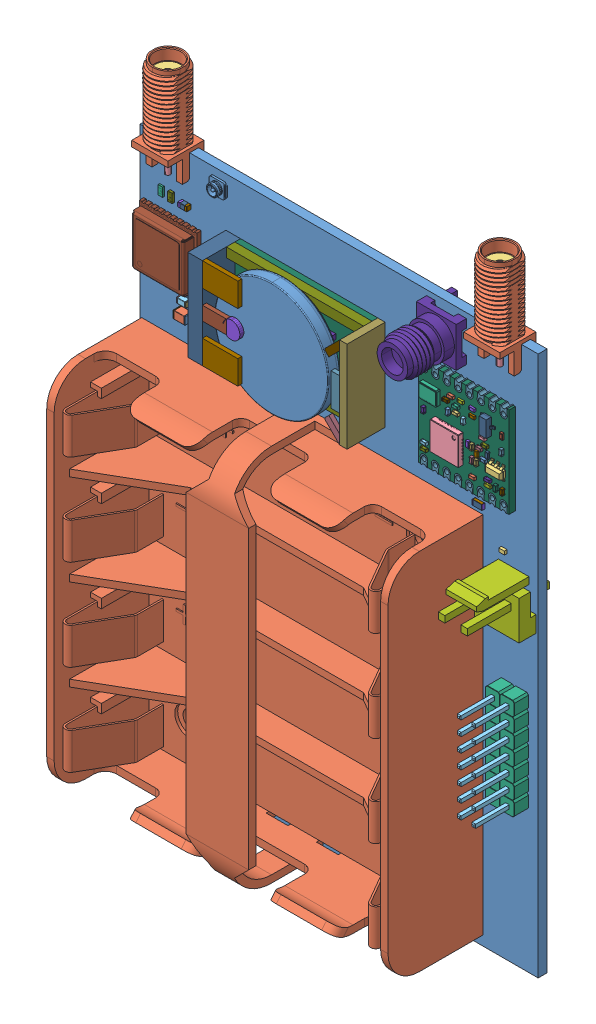
SolidWorks assembly Печатная плата Peggy Tracker, configuration Default. Lengths in mm. (continued)
Components (placement in the parent): (continued)
- Печатная плата Peggy Tracker(2)^Печатная плата Peggy Tracker-1: Печатная плата Peggy Tracker(2)^Печатная плата Peggy Tracker [Default] at origin size (70 108.1 20.64) (virtual) (continued)
  - MPU1^Печатная плата Peggy Tracker(2)_Печатная плата Peggy Tracker-1: MPU1^Печатная плата Peggy Tracker(2)_Печатная плата Peggy Tracker [Default] at origin size (12 12 1.2) (virtual) (continued)
    - 5945464032^MPU1_Печатная плата Peggy Tracker(2)_Печатная плата Peggy Tracker-1: 5945464032^MPU1_Печатная плата Peggy Tracker(2)_Печатная плата Peggy Tracker [Default] at (31.9001 39.0001 -1.5596) x (0 1 0) z (0 0 -1) size (12 12 1.2) (virtual) (continued)
      - Leader^5945464032_MPU1_Печатная плата Peggy Tracker(2)_Печатная плата Peggy Tracker-3: Leader^5945464032_MPU1_Печатная плата Peggy Tracker(2)_Печатная плата Peggy Tracker [По умолчанию] at (-5 -2.4 0) x (-1 0 0) z (0 0 1) size (1 0.38 0.68) (virtual)
      - Leader^5945464032_MPU1_Печатная плата Peggy Tracker(2)_Печатная плата Peggy Tracker-4: Leader^5945464032_MPU1_Печатная плата Peggy Tracker(2)_Печатная плата Peggy Tracker [По умолчанию] at (-5 -1.6 0) x (-1 0 0) z (0 0 1) size (1 0.38 0.68) (virtual)
      - Leader^5945464032_MPU1_Печатная плата Peggy Tracker(2)_Печатная плата Peggy Tracker-5: Leader^5945464032_MPU1_Печатная плата Peggy Tracker(2)_Печатная плата Peggy Tracker [По умолчанию] at (-5 -0.8 0) x (-1 0 0) z (0 0 1) size (1 0.38 0.68) (virtual)
      - Leader^5945464032_MPU1_Печатная плата Peggy Tracker(2)_Печатная плата Peggy Tracker-6: Leader^5945464032_MPU1_Печатная плата Peggy Tracker(2)_Печатная плата Peggy Tracker [По умолчанию] at (-5 0 0) x (-1 0 0) z (0 0 1) size (1 0.38 0.68) (virtual)
      - Leader^5945464032_MPU1_Печатная плата Peggy Tracker(2)_Печатная плата Peggy Tracker-7: Leader^5945464032_MPU1_Печатная плата Peggy Tracker(2)_Печатная плата Peggy Tracker [По умолчанию] at (-5 0.8 0) x (-1 0 0) z (0 0 1) size (1 0.38 0.68) (virtual)
      - Leader^5945464032_MPU1_Печатная плата Peggy Tracker(2)_Печатная плата Peggy Tracker-8: Leader^5945464032_MPU1_Печатная плата Peggy Tracker(2)_Печатная плата Peggy Tracker [По умолчанию] at (-5 1.6 0) x (-1 0 0) z (0 0 1) size (1 0.38 0.68) (virtual)
      - Leader^5945464032_MPU1_Печатная плата Peggy Tracker(2)_Печатная плата Peggy Tracker-9: Leader^5945464032_MPU1_Печатная плата Peggy Tracker(2)_Печатная плата Peggy Tracker [По умолчанию] at (-5 2.4 0) x (-1 0 0) z (0 0 1) size (1 0.38 0.68) (virtual)
      - Leader^5945464032_MPU1_Печатная плата Peggy Tracker(2)_Печатная плата Peggy Tracker-10: Leader^5945464032_MPU1_Печатная плата Peggy Tracker(2)_Печатная плата Peggy Tracker [По умолчанию] at (-5 3.2 0) x (-1 0 0) z (0 0 1) size (1 0.38 0.68) (virtual)
      - Leader^5945464032_MPU1_Печатная плата Peggy Tracker(2)_Печатная плата Peggy Tracker-11: Leader^5945464032_MPU1_Печатная плата Peggy Tracker(2)_Печатная плата Peggy Tracker [По умолчанию] at (-5 4 0) x (-1 0 0) z (0 0 1) size (1 0.38 0.68) (virtual)
      - Leader^5945464032_MPU1_Печатная плата Peggy Tracker(2)_Печатная плата Peggy Tracker-12: Leader^5945464032_MPU1_Печатная плата Peggy Tracker(2)_Печатная плата Peggy Tracker [По умолчанию] at (5 -4 0) size (1 0.38 0.68) (virtual)
      - Leader^5945464032_MPU1_Печатная плата Peggy Tracker(2)_Печатная плата Peggy Tracker-13: Leader^5945464032_MPU1_Печатная плата Peggy Tracker(2)_Печатная плата Peggy Tracker [По умолчанию] at (5 -3.2 0) size (1 0.38 0.68) (virtual)
      - Leader^5945464032_MPU1_Печатная плата Peggy Tracker(2)_Печатная плата Peggy Tracker-14: Leader^5945464032_MPU1_Печатная плата Peggy Tracker(2)_Печатная плата Peggy Tracker [По умолчанию] at (5 -2.4 0) size (1 0.38 0.68) (virtual)
      - Leader^5945464032_MPU1_Печатная плата Peggy Tracker(2)_Печатная плата Peggy Tracker-15: Leader^5945464032_MPU1_Печатная плата Peggy Tracker(2)_Печатная плата Peggy Tracker [По умолчанию] at (5 -1.6 0) size (1 0.38 0.68) (virtual)
      - Leader^5945464032_MPU1_Печатная плата Peggy Tracker(2)_Печатная плата Peggy Tracker-16: Leader^5945464032_MPU1_Печатная плата Peggy Tracker(2)_Печатная плата Peggy Tracker [По умолчанию] at (5 -0.8 0) size (1 0.38 0.68) (virtual)
      - Leader^5945464032_MPU1_Печатная плата Peggy Tracker(2)_Печатная плата Peggy Tracker-17: Leader^5945464032_MPU1_Печатная плата Peggy Tracker(2)_Печатная плата Peggy Tracker [По умолчанию] at (5 0 0) size (1 0.38 0.68) (virtual)
      - Leader^5945464032_MPU1_Печатная плата Peggy Tracker(2)_Печатная плата Peggy Tracker-18: Leader^5945464032_MPU1_Печатная плата Peggy Tracker(2)_Печатная плата Peggy Tracker [По умолчанию] at (5 0.8 0) size (1 0.38 0.68) (virtual)
      - Leader^5945464032_MPU1_Печатная плата Peggy Tracker(2)_Печатная плата Peggy Tracker-19: Leader^5945464032_MPU1_Печатная плата Peggy Tracker(2)_Печатная плата Peggy Tracker [По умолчанию] at (5 1.6 0) size (1 0.38 0.68) (virtual)
      - Leader^5945464032_MPU1_Печатная плата Peggy Tracker(2)_Печатная плата Peggy Tracker-20: Leader^5945464032_MPU1_Печатная плата Peggy Tracker(2)_Печатная плата Peggy Tracker [По умолчанию] at (5 2.4 0) size (1 0.38 0.68) (virtual)
      - Leader^5945464032_MPU1_Печатная плата Peggy Tracker(2)_Печатная плата Peggy Tracker-21: Leader^5945464032_MPU1_Печатная плата Peggy Tracker(2)_Печатная плата Peggy Tracker [По умолчанию] at (5 3.2 0) size (1 0.38 0.68) (virtual)
      - Leader^5945464032_MPU1_Печатная плата Peggy Tracker(2)_Печатная плата Peggy Tracker-22: Leader^5945464032_MPU1_Печатная плата Peggy Tracker(2)_Печатная плата Peggy Tracker [По умолчанию] at (5 4 0) size (1 0.38 0.68) (virtual)
      - Leader-13^5945464032_MPU1_Печатная плата Peggy Tracker(2)_Печатная плата Peggy Tracker-1: Leader-13^5945464032_MPU1_Печатная плата Peggy Tracker(2)_Печатная плата Peggy Tracker [По умолчанию] at (-4 -5 0) x (0 -1 0) z (0 0 1) size (1 0.38 0.68) (virtual)
      - Leader-13^5945464032_MPU1_Печатная плата Peggy Tracker(2)_Печатная плата Peggy Tracker-2: Leader-13^5945464032_MPU1_Печатная плата Peggy Tracker(2)_Печатная плата Peggy Tracker [По умолчанию] at (-3.2 -5 0) x (0 -1 0) z (0 0 1) size (1 0.38 0.68) (virtual)
      - Leader-13^5945464032_MPU1_Печатная плата Peggy Tracker(2)_Печатная плата Peggy Tracker-3: Leader-13^5945464032_MPU1_Печатная плата Peggy Tracker(2)_Печатная плата Peggy Tracker [По умолчанию] at (-2.4 -5 0) x (0 -1 0) z (0 0 1) size (1 0.38 0.68) (virtual)
      - Leader-13^5945464032_MPU1_Печатная плата Peggy Tracker(2)_Печатная плата Peggy Tracker-4: Leader-13^5945464032_MPU1_Печатная плата Peggy Tracker(2)_Печатная плата Peggy Tracker [По умолчанию] at (-1.6 -5 0) x (0 -1 0) z (0 0 1) size (1 0.38 0.68) (virtual)
      - Leader-13^5945464032_MPU1_Печатная плата Peggy Tracker(2)_Печатная плата Peggy Tracker-5: Leader-13^5945464032_MPU1_Печатная плата Peggy Tracker(2)_Печатная плата Peggy Tracker [По умолчанию] at (-0.8 -5 0) x (0 -1 0) z (0 0 1) size (1 0.38 0.68) (virtual)
      - Leader-13^5945464032_MPU1_Печатная плата Peggy Tracker(2)_Печатная плата Peggy Tracker-6: Leader-13^5945464032_MPU1_Печатная плата Peggy Tracker(2)_Печатная плата Peggy Tracker [По умолчанию] at (0 -5 0) x (0 -1 0) z (0 0 1) size (1 0.38 0.68) (virtual)
      - Leader-13^5945464032_MPU1_Печатная плата Peggy Tracker(2)_Печатная плата Peggy Tracker-7: Leader-13^5945464032_MPU1_Печатная плата Peggy Tracker(2)_Печатная плата Peggy Tracker [По умолчанию] at (0.8 -5 0) x (0 -1 0) z (0 0 1) size (1 0.38 0.68) (virtual)
      - Leader-13^5945464032_MPU1_Печатная плата Peggy Tracker(2)_Печатная плата Peggy Tracker-8: Leader-13^5945464032_MPU1_Печатная плата Peggy Tracker(2)_Печатная плата Peggy Tracker [По умолчанию] at (1.6 -5 0) x (0 -1 0) z (0 0 1) size (1 0.38 0.68) (virtual)
      - Leader-13^5945464032_MPU1_Печатная плата Peggy Tracker(2)_Печатная плата Peggy Tracker-9: Leader-13^5945464032_MPU1_Печатная плата Peggy Tracker(2)_Печатная плата Peggy Tracker [По умолчанию] at (2.4 -5 0) x (0 -1 0) z (0 0 1) size (1 0.38 0.68) (virtual)
      - Leader-13^5945464032_MPU1_Печатная плата Peggy Tracker(2)_Печатная плата Peggy Tracker-10: Leader-13^5945464032_MPU1_Печатная плата Peggy Tracker(2)_Печатная плата Peggy Tracker [По умолчанию] at (3.2 -5 0) x (0 -1 0) z (0 0 1) size (1 0.38 0.68) (virtual)
      - Leader-13^5945464032_MPU1_Печатная плата Peggy Tracker(2)_Печатная плата Peggy Tracker-11: Leader-13^5945464032_MPU1_Печатная плата Peggy Tracker(2)_Печатная плата Peggy Tracker [По умолчанию] at (4 -5 0) x (0 -1 0) z (0 0 1) size (1 0.38 0.68) (virtual)
      - Leader-13^5945464032_MPU1_Печатная плата Peggy Tracker(2)_Печатная плата Peggy Tracker-12: Leader-13^5945464032_MPU1_Печатная плата Peggy Tracker(2)_Печатная плата Peggy Tracker [По умолчанию] at (-4 5 0) x (0 1 0) z (0 0 1) size (1 0.38 0.68) (virtual)
      - Leader-13^5945464032_MPU1_Печатная плата Peggy Tracker(2)_Печатная плата Peggy Tracker-13: Leader-13^5945464032_MPU1_Печатная плата Peggy Tracker(2)_Печатная плата Peggy Tracker [По умолчанию] at (-3.2 5 0) x (0 1 0) z (0 0 1) size (1 0.38 0.68) (virtual)
      - Leader-13^5945464032_MPU1_Печатная плата Peggy Tracker(2)_Печатная плата Peggy Tracker-14: Leader-13^5945464032_MPU1_Печатная плата Peggy Tracker(2)_Печатная плата Peggy Tracker [По умолчанию] at (-2.4 5 0) x (0 1 0) z (0 0 1) size (1 0.38 0.68) (virtual)
      - Leader-13^5945464032_MPU1_Печатная плата Peggy Tracker(2)_Печатная плата Peggy Tracker-15: Leader-13^5945464032_MPU1_Печатная плата Peggy Tracker(2)_Печатная плата Peggy Tracker [По умолчанию] at (-1.6 5 0) x (0 1 0) z (0 0 1) size (1 0.38 0.68) (virtual)
      - Leader-13^5945464032_MPU1_Печатная плата Peggy Tracker(2)_Печатная плата Peggy Tracker-16: Leader-13^5945464032_MPU1_Печатная плата Peggy Tracker(2)_Печатная плата Peggy Tracker [По умолчанию] at (-0.8 5 0) x (0 1 0) z (0 0 1) size (1 0.38 0.68) (virtual)
      - Leader-13^5945464032_MPU1_Печатная плата Peggy Tracker(2)_Печатная плата Peggy Tracker-17: Leader-13^5945464032_MPU1_Печатная плата Peggy Tracker(2)_Печатная плата Peggy Tracker [По умолчанию] at (0 5 0) x (0 1 0) z (0 0 1) size (1 0.38 0.68) (virtual)
      - Leader-13^5945464032_MPU1_Печатная плата Peggy Tracker(2)_Печатная плата Peggy Tracker-18: Leader-13^5945464032_MPU1_Печатная плата Peggy Tracker(2)_Печатная плата Peggy Tracker [По умолчанию] at (0.8 5 0) x (0 1 0) z (0 0 1) size (1 0.38 0.68) (virtual)
      - Leader-13^5945464032_MPU1_Печатная плата Peggy Tracker(2)_Печатная плата Peggy Tracker-19: Leader-13^5945464032_MPU1_Печатная плата Peggy Tracker(2)_Печатная плата Peggy Tracker [По умолчанию] at (1.6 5 0) x (0 1 0) z (0 0 1) size (1 0.38 0.68) (virtual)
      - Leader-13^5945464032_MPU1_Печатная плата Peggy Tracker(2)_Печатная плата Peggy Tracker-20: Leader-13^5945464032_MPU1_Печатная плата Peggy Tracker(2)_Печатная плата Peggy Tracker [По умолчанию] at (2.4 5 0) x (0 1 0) z (0 0 1) size (1 0.38 0.68) (virtual)
      - Leader-13^5945464032_MPU1_Печатная плата Peggy Tracker(2)_Печатная плата Peggy Tracker-21: Leader-13^5945464032_MPU1_Печатная плата Peggy Tracker(2)_Печатная плата Peggy Tracker [По умолчанию] at (3.2 5 0) x (0 1 0) z (0 0 1) size (1 0.38 0.68) (virtual)
      - Leader-13^5945464032_MPU1_Печатная плата Peggy Tracker(2)_Печатная плата Peggy Tracker-22: Leader-13^5945464032_MPU1_Печатная плата Peggy Tracker(2)_Печатная плата Peggy Tracker [По умолчанию] at (4 5 0) x (0 1 0) z (0 0 1) size (1 0.38 0.68) (virtual)
    - User_Library-VQFN(44)^MPU1_Печатная плата Peggy Tracker(2)_Печатная плата Peggy Tracker-1: User_Library-VQFN(44)^MPU1_Печатная плата Peggy Tracker(2)_Печатная плата Peggy Tracker [По умолчанию] at (28.3541 42.5231 -1.5596) x (1 0 0) z (0 1 0) size (7.1 0.95 7.1) (virtual)
  - L3^Печатная плата Peggy Tracker(2)_Печатная плата Peggy Tracker-1: L3^Печатная плата Peggy Tracker(2)_Печатная плата Peggy Tracker [Default] at origin size (1.25 2 0.85) (virtual)
    - User_Library-FB_2012-1^L3_Печатная плата Peggy Tracker(2)_Печатная плата Peggy Tracker-1: User_Library-FB_2012-1^L3_Печатная плата Peggy Tracker(2)_Печатная плата Peggy Tracker [Default] at (29.1001 21.7001 -1.5596) x (0 1 0) z (0 0 -1) size (2 1.25 0.85) (virtual)
      - User_Library-FB_2012-1_Pad001^User_Library-FB_2012-1_L3_Печатная плата Peggy Tracker(2)_Печатная плата Peggy Tracker-1: User_Library-FB_2012-1_Pad001^User_Library-FB_2012-1_L3_Печатная плата Peggy Tracker(2)_Печатная плата Peggy Tracker [По умолчанию] at (0 0 0.03) size (1.94 1.19 0.79) (virtual)
      - User_Library-FB_2012-1_Cut^User_Library-FB_2012-1_L3_Печатная плата Peggy Tracker(2)_Печатная плата Peggy Tracker-1: User_Library-FB_2012-1_Cut^User_Library-FB_2012-1_L3_Печатная плата Peggy Tracker(2)_Печатная плата Peggy Tracker [По умолчанию] at origin size (2 1.25 0.85) (virtual)
  - L2^Печатная плата Peggy Tracker(2)_Печатная плата Peggy Tracker-1: L2^Печатная плата Peggy Tracker(2)_Печатная плата Peggy Tracker [Default] at origin size (2 1.25 0.85) (virtual)
    - User_Library-FB_2012-1^L2_Печатная плата Peggy Tracker(2)_Печатная плата Peggy Tracker-1: User_Library-FB_2012-1^L2_Печатная плата Peggy Tracker(2)_Печатная плата Peggy Tracker [Default] at (56.1999 81.8001 -1.5596) x (-1 0 0) z (0 0 -1) size (2 1.25 0.85) (virtual)
      - User_Library-FB_2012-1_Pad001^User_Library-FB_2012-1_L2_Печатная плата Peggy Tracker(2)_Печатная плата Peggy Tracker-1: User_Library-FB_2012-1_Pad001^User_Library-FB_2012-1_L2_Печатная плата Peggy Tracker(2)_Печатная плата Peggy Tracker [По умолчанию] at (0 0 0.03) size (1.94 1.19 0.79) (virtual)
      - User_Library-FB_2012-1_Cut^User_Library-FB_2012-1_L2_Печатная плата Peggy Tracker(2)_Печатная плата Peggy Tracker-1: User_Library-FB_2012-1_Cut^User_Library-FB_2012-1_L2_Печатная плата Peggy Tracker(2)_Печатная плата Peggy Tracker [По умолчанию] at origin size (2 1.25 0.85) (virtual)
  - L1^Печатная плата Peggy Tracker(2)_Печатная плата Peggy Tracker-1: L1^Печатная плата Peggy Tracker(2)_Печатная плата Peggy Tracker [Default] at origin size (1.6 0.8 0.8) (virtual)
    - 5945464832^L1_Печатная плата Peggy Tracker(2)_Печатная плата Peggy Tracker-1: 5945464832^L1_Печатная плата Peggy Tracker(2)_Печатная плата Peggy Tracker [Default] at (8.2 86.9 0) size (1.6 0.8 0.8) (virtual)
      - Terminal-2^5945464832_L1_Печатная плата Peggy Tracker(2)_Печатная плата Peggy Tracker-1: Terminal-2^5945464832_L1_Печатная плата Peggy Tracker(2)_Печатная плата Peggy Tracker [Default] at (-0.8 -0.4 0) size (1.6 0.8 0.8) (virtual)
        - Open_CASCADE_STEP_translator_6.8_17.1.1^Terminal-2_5945464832_L1_Печатная плата Peggy Tracker(2)_Печатная плата Peggy Tracker-1: Open_CASCADE_STEP_translator_6.8_17.1.1^Terminal-2_5945464832_L1_Печатная плата Peggy Tracker(2)_Печатная плата Peggy Tracker [По умолчанию] at origin size (0.4 0.8 0.8) (virtual)
        - Open_CASCADE_STEP_translator_6.8_17.1.2^Terminal-2_5945464832_L1_Печатная плата Peggy Tracker(2)_Печатная плата Peggy Tracker-1: Open_CASCADE_STEP_translator_6.8_17.1.2^Terminal-2_5945464832_L1_Печатная плата Peggy Tracker(2)_Печатная плата Peggy Tracker [По умолчанию] at origin size (0.4 0.8 0.8) (virtual)
      - Mid_Body-14^5945464832_L1_Печатная плата Peggy Tracker(2)_Печатная плата Peggy Tracker-1: Mid_Body-14^5945464832_L1_Печатная плата Peggy Tracker(2)_Печатная плата Peggy Tracker [Default] at (-0.8 -0.4 0) size (0.8 0.8 0.8) (virtual)
        - Open_CASCADE_STEP_translator_6.8_17.2.1^Mid_Body-14_5945464832_L1_Печатная плата Peggy Tracker(2)_Печатная плата Peggy Tracker-1: Open_CASCADE_STEP_translator_6.8_17.2.1^Mid_Body-14_5945464832_L1_Печатная плата Peggy Tracker(2)_Печатная плата Peggy Tracker [По умолчанию] at origin size (0.8 0.8 0.8) (virtual)
  - HL1^Печатная плата Peggy Tracker(2)_Печатная плата Peggy Tracker-1: HL1^Печатная плата Peggy Tracker(2)_Печатная плата Peggy Tracker [Default] at origin size (0.81 1.61 0.61) (virtual)
    - User_Library-LED_0603_G^HL1_Печатная плата Peggy Tracker(2)_Печатная плата Peggy Tracker-1: User_Library-LED_0603_G^HL1_Печатная плата Peggy Tracker(2)_Печатная плата Peggy Tracker [Default] at (37.1999 47.7999 -1.5596) x (0 -1 0) z (0 0 -1) size (1.61 0.81 0.61) (virtual)
      - User_Library-LED_0603_G_Pocket002^User_Library-LED_0603_G_HL1_Печатная плата Peggy Tracker(2)_Печатная плата Peggy Tracker-1: User_Library-LED_0603_G_Pocket002^User_Library-LED_0603_G_HL1_Печатная плата Peggy Tracker(2)_Печатная плата Peggy Tracker [По умолчанию] at origin size (0.41 0.81 0.21) (virtual)
      - User_Library-LED_0603_G_Pad004^User_Library-LED_0603_G_HL1_Печатная плата Peggy Tracker(2)_Печатная плата Peggy Tracker-1: User_Library-LED_0603_G_Pad004^User_Library-LED_0603_G_HL1_Печатная плата Peggy Tracker(2)_Печатная плата Peggy Tracker [По умолчанию] x (1 0 0) z (0 0 -1) size (0.4 0.8 0) (virtual)
      - User_Library-LED_0603_G_Fillet^User_Library-LED_0603_G_HL1_Печатная плата Peggy Tracker(2)_Печатная плата Peggy Tracker-1: User_Library-LED_0603_G_Fillet^User_Library-LED_0603_G_HL1_Печатная плата Peggy Tracker(2)_Печатная плата Peggy Tracker [По умолчанию] at origin size (1 0.7 0.4) (virtual)
      - User_Library-LED_0603_G_Pocket001^User_Library-LED_0603_G_HL1_Печатная плата Peggy Tracker(2)_Печатная плата Peggy Tracker-1: User_Library-LED_0603_G_Pocket001^User_Library-LED_0603_G_HL1_Печатная плата Peggy Tracker(2)_Печатная плата Peggy Tracker [По умолчанию] at origin size (0.4 0.8 0.2) (virtual)
      - User_Library-LED_0603_G_Pad^User_Library-LED_0603_G_HL1_Печатная плата Peggy Tracker(2)_Печатная плата Peggy Tracker-1: User_Library-LED_0603_G_Pad^User_Library-LED_0603_G_HL1_Печатная плата Peggy Tracker(2)_Печатная плата Peggy Tracker [По умолчанию] at origin size (0.8 0.8 0.2) (virtual)
  - DD2^Печатная плата Peggy Tracker(2)_Печатная плата Peggy Tracker-1: DD2^Печатная плата Peggy Tracker(2)_Печатная плата Peggy Tracker [Default] at origin size (15.9 16 2.23) (virtual)
    - User_Library-RFM96W^DD2_Печатная плата Peggy Tracker(2)_Печатная плата Peggy Tracker-1: User_Library-RFM96W^DD2_Печатная плата Peggy Tracker(2)_Печатная плата Peggy Tracker [Default] at (50.075 85.102 1.15) x (0 -1 0) z (0 0 1) size (16 15.9 2.23) (virtual)
      - Designator4^User_Library-RFM96W_DD2_Печатная плата Peggy Tracker(2)_Печатная плата Peggy Tracker-1: Designator4^User_Library-RFM96W_DD2_Печатная плата Peggy Tracker(2)_Печатная плата Peggy Tracker [Default] at origin size (0.5 1 0.5) (virtual)
        - Cap0402^Designator4_User_Library-RFM96W_DD2_Печатная плата Peggy Tracker(2)_Печатная плата Peggy Tracker-1: Cap0402^Designator4_User_Library-RFM96W_DD2_Печатная плата Peggy Tracker(2)_Печатная плата Peggy Tracker [По умолчанию] at (13.208 1.27 0) x (0 -1 0) z (-1 0 0) size (1 0.5 0.5) (virtual)
      - Designator6^User_Library-RFM96W_DD2_Печатная плата Peggy Tracker(2)_Печатная плата Peggy Tracker-1: Designator6^User_Library-RFM96W_DD2_Печатная плата Peggy Tracker(2)_Печатная плата Peggy Tracker [Default] at origin size (1 0.5 0.5) (virtual)
        - Cap0402^Designator6_User_Library-RFM96W_DD2_Печатная плата Peggy Tracker(2)_Печатная плата Peggy Tracker-1: Cap0402^Designator6_User_Library-RFM96W_DD2_Печатная плата Peggy Tracker(2)_Печатная плата Peggy Tracker [По умолчанию] at (7.239 1.143 0) x (-1 0 0) z (0 1 0) size (1 0.5 0.5) (virtual)
      - Designator7^User_Library-RFM96W_DD2_Печатная плата Peggy Tracker(2)_Печатная плата Peggy Tracker-1: Designator7^User_Library-RFM96W_DD2_Печатная плата Peggy Tracker(2)_Печатная плата Peggy Tracker [Default] at origin size (0.5 1 0.5) (virtual)
        - Cap0402^Designator7_User_Library-RFM96W_DD2_Печатная плата Peggy Tracker(2)_Печатная плата Peggy Tracker-1: Cap0402^Designator7_User_Library-RFM96W_DD2_Печатная плата Peggy Tracker(2)_Печатная плата Peggy Tracker [По умолчанию] at (3.81 5.08 0) x (0 -1 0) z (-1 0 0) size (1 0.5 0.5) (virtual)
      - Designator8^User_Library-RFM96W_DD2_Печатная плата Peggy Tracker(2)_Печатная плата Peggy Tracker-1: Designator8^User_Library-RFM96W_DD2_Печатная плата Peggy Tracker(2)_Печатная плата Peggy Tracker [Default] at origin size (1 0.5 0.5) (virtual)
        - Cap0402^Designator8_User_Library-RFM96W_DD2_Печатная плата Peggy Tracker(2)_Печатная плата Peggy Tracker-1: Cap0402^Designator8_User_Library-RFM96W_DD2_Печатная плата Peggy Tracker(2)_Печатная плата Peggy Tracker [По умолчанию] at (5.4 5.45 0) x (1 0 0) z (0 -1 0) size (1 0.5 0.5) (virtual)
      - Designator9^User_Library-RFM96W_DD2_Печатная плата Peggy Tracker(2)_Печатная плата Peggy Tracker-1: Designator9^User_Library-RFM96W_DD2_Печатная плата Peggy Tracker(2)_Печатная плата Peggy Tracker [Default] at origin size (0.5 1 0.5) (virtual)
        - Cap0402^Designator9_User_Library-RFM96W_DD2_Печатная плата Peggy Tracker(2)_Печатная плата Peggy Tracker-1: Cap0402^Designator9_User_Library-RFM96W_DD2_Печатная плата Peggy Tracker(2)_Печатная плата Peggy Tracker [По умолчанию] at (2.8 5.98 0) x (0 -1 0) z (-1 0 0) size (1 0.5 0.5) (virtual)
      - Designator10^User_Library-RFM96W_DD2_Печатная плата Peggy Tracker(2)_Печатная плата Peggy Tracker-1: Designator10^User_Library-RFM96W_DD2_Печатная плата Peggy Tracker(2)_Печатная плата Peggy Tracker [Default] at origin size (0.5 1 0.5) (virtual)
        - Cap0402^Designator10_User_Library-RFM96W_DD2_Печатная плата Peggy Tracker(2)_Печатная плата Peggy Tracker-1: Cap0402^Designator10_User_Library-RFM96W_DD2_Печатная плата Peggy Tracker(2)_Печатная плата Peggy Tracker [По умолчанию] at (4.953 6.858 0) x (0 -1 0) z (-1 0 0) size (1 0.5 0.5) (virtual)
      - Designator11^User_Library-RFM96W_DD2_Печатная плата Peggy Tracker(2)_Печатная плата Peggy Tracker-1: Designator11^User_Library-RFM96W_DD2_Печатная плата Peggy Tracker(2)_Печатная плата Peggy Tracker [Default] at origin size (0.5 1 0.5) (virtual)
        - Cap0402^Designator11_User_Library-RFM96W_DD2_Печатная плата Peggy Tracker(2)_Печатная плата Peggy Tracker-1: Cap0402^Designator11_User_Library-RFM96W_DD2_Печатная плата Peggy Tracker(2)_Печатная плата Peggy Tracker [По умолчанию] at (6.35 11.557 0) x (0 1 0) z (1 0 0) size (1 0.5 0.5) (virtual)
      - Designator12^User_Library-RFM96W_DD2_Печатная плата Peggy Tracker(2)_Печатная плата Peggy Tracker-1: Designator12^User_Library-RFM96W_DD2_Печатная плата Peggy Tracker(2)_Печатная плата Peggy Tracker [Default] at origin size (1 0.5 0.5) (virtual)
        - Cap0402^Designator12_User_Library-RFM96W_DD2_Печатная плата Peggy Tracker(2)_Печатная плата Peggy Tracker-1: Cap0402^Designator12_User_Library-RFM96W_DD2_Печатная плата Peggy Tracker(2)_Печатная плата Peggy Tracker [По умолчанию] at (5.461 8.128 0) x (1 0 0) z (0 -1 0) size (1 0.5 0.5) (virtual)
      - Designator13^User_Library-RFM96W_DD2_Печатная плата Peggy Tracker(2)_Печатная плата Peggy Tracker-1: Designator13^User_Library-RFM96W_DD2_Печатная плата Peggy Tracker(2)_Печатная плата Peggy Tracker [Default] at origin size (0.5 1 0.5) (virtual)
        - Cap0402^Designator13_User_Library-RFM96W_DD2_Печатная плата Peggy Tracker(2)_Печатная плата Peggy Tracker-1: Cap0402^Designator13_User_Library-RFM96W_DD2_Печатная плата Peggy Tracker(2)_Печатная плата Peggy Tracker [По умолчанию] at (3.937 6.858 0) x (0 1 0) z (1 0 0) size (1 0.5 0.5) (virtual)
      - Designator15^User_Library-RFM96W_DD2_Печатная плата Peggy Tracker(2)_Печатная плата Peggy Tracker-1: Designator15^User_Library-RFM96W_DD2_Печатная плата Peggy Tracker(2)_Печатная плата Peggy Tracker [Default] at origin size (0.52 1.02 0.37) (virtual)
        - SW3dPS-inductor_0402_white^Designator15_User_Library-RFM96W_DD2_Печатная плата Peggy Tracker(2)_Печатная плата Peggy Tracker-1: SW3dPS-inductor_0402_white^Designator15_User_Library-RFM96W_DD2_Печатная плата Peggy Tracker(2)_Печатная плата Peggy Tracker [По умолчанию] at (13.208 12.446 0) x (1 0 0) z (0 -1 0) size (0.52 0.37 1.02) (virtual)
      - Designator17^User_Library-RFM96W_DD2_Печатная плата Peggy Tracker(2)_Печатная плата Peggy Tracker-1: Designator17^User_Library-RFM96W_DD2_Печатная плата Peggy Tracker(2)_Печатная плата Peggy Tracker [Default] at origin size (1.02 0.52 0.37) (virtual)
        - SW3dPS-inductor_0402_white^Designator17_User_Library-RFM96W_DD2_Печатная плата Peggy Tracker(2)_Печатная плата Peggy Tracker-1: SW3dPS-inductor_0402_white^Designator17_User_Library-RFM96W_DD2_Печатная плата Peggy Tracker(2)_Печатная плата Peggy Tracker [По умолчанию] at (8.636 8.89 0) x (0 1 0) z (1 0 0) size (0.52 0.37 1.02) (virtual)
      - Designator18^User_Library-RFM96W_DD2_Печатная плата Peggy Tracker(2)_Печатная плата Peggy Tracker-1: Designator18^User_Library-RFM96W_DD2_Печатная плата Peggy Tracker(2)_Печатная плата Peggy Tracker [Default] at origin size (1.02 0.52 0.37) (virtual)
        - SW3dPS-inductor_0402_white^Designator18_User_Library-RFM96W_DD2_Печатная плата Peggy Tracker(2)_Печатная плата Peggy Tracker-1: SW3dPS-inductor_0402_white^Designator18_User_Library-RFM96W_DD2_Печатная плата Peggy Tracker(2)_Печатная плата Peggy Tracker [По умолчанию] at (9.398 10.414 0) x (0 1 0) z (1 0 0) size (0.52 0.37 1.02) (virtual)
      - Designator19^User_Library-RFM96W_DD2_Печатная плата Peggy Tracker(2)_Печатная плата Peggy Tracker-1: Designator19^User_Library-RFM96W_DD2_Печатная плата Peggy Tracker(2)_Печатная плата Peggy Tracker [Default] at origin size (1.02 0.52 0.37) (virtual)
        - SW3dPS-inductor_0402_white^Designator19_User_Library-RFM96W_DD2_Печатная плата Peggy Tracker(2)_Печатная плата Peggy Tracker-1: SW3dPS-inductor_0402_white^Designator19_User_Library-RFM96W_DD2_Печатная плата Peggy Tracker(2)_Печатная плата Peggy Tracker [По умолчанию] at (8.636 12.319 0) x (0 1 0) z (1 0 0) size (0.52 0.37 1.02) (virtual)
      - Designator20^User_Library-RFM96W_DD2_Печатная плата Peggy Tracker(2)_Печатная плата Peggy Tracker-1: Designator20^User_Library-RFM96W_DD2_Печатная плата Peggy Tracker(2)_Печатная плата Peggy Tracker [Default] at origin size (1.02 0.52 0.37) (virtual)
        - SW3dPS-inductor_0402_white^Designator20_User_Library-RFM96W_DD2_Печатная плата Peggy Tracker(2)_Печатная плата Peggy Tracker-1: SW3dPS-inductor_0402_white^Designator20_User_Library-RFM96W_DD2_Печатная плата Peggy Tracker(2)_Печатная плата Peggy Tracker [По умолчанию] at (10.668 12.319 0) x (0 1 0) z (1 0 0) size (0.52 0.37 1.02) (virtual)
      - Designator21^User_Library-RFM96W_DD2_Печатная плата Peggy Tracker(2)_Печатная плата Peggy Tracker-1: Designator21^User_Library-RFM96W_DD2_Печатная плата Peggy Tracker(2)_Печатная плата Peggy Tracker [Default] at origin size (1 0.5 0.5) (virtual)
        - Cap0402^Designator21_User_Library-RFM96W_DD2_Печатная плата Peggy Tracker(2)_Печатная плата Peggy Tracker-1: Cap0402^Designator21_User_Library-RFM96W_DD2_Печатная плата Peggy Tracker(2)_Печатная плата Peggy Tracker [По умолчанию] at (10.668 10.414 0) x (-1 0 0) z (0 1 0) size (1 0.5 0.5) (virtual)
      - Designator22^User_Library-RFM96W_DD2_Печатная плата Peggy Tracker(2)_Печатная плата Peggy Tracker-1: Designator22^User_Library-RFM96W_DD2_Печатная плата Peggy Tracker(2)_Печатная плата Peggy Tracker [Default] at origin size (0.5 1 0.5) (virtual)
        - Cap0402^Designator22_User_Library-RFM96W_DD2_Печатная плата Peggy Tracker(2)_Печатная плата Peggy Tracker-1: Cap0402^Designator22_User_Library-RFM96W_DD2_Печатная плата Peggy Tracker(2)_Печатная плата Peggy Tracker [По умолчанию] at (8.255 10.922 0) x (0 1 0) z (1 0 0) size (1 0.5 0.5) (virtual)
      - Designator23^User_Library-RFM96W_DD2_Печатная плата Peggy Tracker(2)_Печатная плата Peggy Tracker-1: Designator23^User_Library-RFM96W_DD2_Печатная плата Peggy Tracker(2)_Печатная плата Peggy Tracker [Default] at origin size (1 0.5 0.5) (virtual)
        - Cap0402^Designator23_User_Library-RFM96W_DD2_Печатная плата Peggy Tracker(2)_Печатная плата Peggy Tracker-1: Cap0402^Designator23_User_Library-RFM96W_DD2_Печатная плата Peggy Tracker(2)_Печатная плата Peggy Tracker [По умолчанию] at (6.858 14.859 0) x (-1 0 0) z (0 1 0) size (1 0.5 0.5) (virtual)
      - Designator24^User_Library-RFM96W_DD2_Печатная плата Peggy Tracker(2)_Печатная плата Peggy Tracker-1: Designator24^User_Library-RFM96W_DD2_Печатная плата Peggy Tracker(2)_Печатная плата Peggy Tracker [Default] at origin size (1 0.5 0.5) (virtual)
        - Cap0402^Designator24_User_Library-RFM96W_DD2_Печатная плата Peggy Tracker(2)_Печатная плата Peggy Tracker-1: Cap0402^Designator24_User_Library-RFM96W_DD2_Печатная плата Peggy Tracker(2)_Печатная плата Peggy Tracker [По умолчанию] at (12.827 13.843 0) x (-1 0 0) z (0 1 0) size (1 0.5 0.5) (virtual)
      - Designator25^User_Library-RFM96W_DD2_Печатная плата Peggy Tracker(2)_Печатная плата Peggy Tracker-1: Designator25^User_Library-RFM96W_DD2_Печатная плата Peggy Tracker(2)_Печатная плата Peggy Tracker [Default] at origin size (0.5 1 0.5) (virtual)
        - Cap0402^Designator25_User_Library-RFM96W_DD2_Печатная плата Peggy Tracker(2)_Печатная плата Peggy Tracker-1: Cap0402^Designator25_User_Library-RFM96W_DD2_Печатная плата Peggy Tracker(2)_Печатная плата Peggy Tracker [По умолчанию] at (7.366 11.938 0) x (0 -1 0) z (-1 0 0) size (1 0.5 0.5) (virtual)
      - Designator26^User_Library-RFM96W_DD2_Печатная плата Peggy Tracker(2)_Печатная плата Peggy Tracker-1: Designator26^User_Library-RFM96W_DD2_Печатная плата Peggy Tracker(2)_Печатная плата Peggy Tracker [Default] at origin size (0.5 1 0.5) (virtual)
        - Cap0402^Designator26_User_Library-RFM96W_DD2_Печатная плата Peggy Tracker(2)_Печатная плата Peggy Tracker-1: Cap0402^Designator26_User_Library-RFM96W_DD2_Печатная плата Peggy Tracker(2)_Печатная плата Peggy Tracker [По умолчанию] at (12.319 12.446 0) x (0 -1 0) z (-1 0 0) size (1 0.5 0.5) (virtual)
      - Designator27^User_Library-RFM96W_DD2_Печатная плата Peggy Tracker(2)_Печатная плата Peggy Tracker-1: Designator27^User_Library-RFM96W_DD2_Печатная плата Peggy Tracker(2)_Печатная плата Peggy Tracker [Default] at origin size (1 0.5 0.5) (virtual)
        - Cap0402^Designator27_User_Library-RFM96W_DD2_Печатная плата Peggy Tracker(2)_Печатная плата Peggy Tracker-1: Cap0402^Designator27_User_Library-RFM96W_DD2_Печатная плата Peggy Tracker(2)_Печатная плата Peggy Tracker [По умолчанию] at (12.827 14.986 0) x (-1 0 0) z (0 1 0) size (1 0.5 0.5) (virtual)
      - Designator28^User_Library-RFM96W_DD2_Печатная плата Peggy Tracker(2)_Печатная плата Peggy Tracker-1: Designator28^User_Library-RFM96W_DD2_Печатная плата Peggy Tracker(2)_Печатная плата Peggy Tracker [Default] at origin size (0.5 1 0.5) (virtual)
        - Cap0402^Designator28_User_Library-RFM96W_DD2_Печатная плата Peggy Tracker(2)_Печатная плата Peggy Tracker-1: Cap0402^Designator28_User_Library-RFM96W_DD2_Печатная плата Peggy Tracker(2)_Печатная плата Peggy Tracker [По умолчанию] at (9.652 11.684 0) x (0 -1 0) z (-1 0 0) size (1 0.5 0.5) (virtual)
      - Designator29^User_Library-RFM96W_DD2_Печатная плата Peggy Tracker(2)_Печатная плата Peggy Tracker-1: Designator29^User_Library-RFM96W_DD2_Печатная плата Peggy Tracker(2)_Печатная плата Peggy Tracker [Default] at origin size (0.5 1 0.5) (virtual)
        - Cap0402^Designator29_User_Library-RFM96W_DD2_Печатная плата Peggy Tracker(2)_Печатная плата Peggy Tracker-1: Cap0402^Designator29_User_Library-RFM96W_DD2_Печатная плата Peggy Tracker(2)_Печатная плата Peggy Tracker [По умолчанию] at (13.208 9.779 0) x (0 -1 0) z (-1 0 0) size (1 0.5 0.5) (virtual)
      - Designator27_2^User_Library-RFM96W_DD2_Печатная плата Peggy Tracker(2)_Печатная плата Peggy Tracker-1: Designator27_2^User_Library-RFM96W_DD2_Печатная плата Peggy Tracker(2)_Печатная плата Peggy Tracker [Default] at origin size (2.43 2.79 1.09) (virtual)
        - SW3dPS-SOT-23-6^Designator27_2_User_Library-RFM96W_DD2_Печатная плата Peggy Tracker(2)_Печатная плата Peggy Tracker-1: SW3dPS-SOT-23-6^Designator27_2_User_Library-RFM96W_DD2_Печатная плата Peggy Tracker(2)_Печатная плата Peggy Tracker [По умолчанию] at (9.0742 15.0495 0) x (0 -1 0) z (0 0 1) size (2.79 2.43 1.09) (virtual)
      - Designator2^User_Library-RFM96W_DD2_Печатная плата Peggy Tracker(2)_Печатная плата Peggy Tracker-1: Designator2^User_Library-RFM96W_DD2_Печатная плата Peggy Tracker(2)_Печатная плата Peggy Tracker [Default] at origin size (5.04 5.04 0.9) (virtual)
        - QFN28^Designator2_User_Library-RFM96W_DD2_Печатная плата Peggy Tracker(2)_Печатная плата Peggy Tracker-1: QFN28^Designator2_User_Library-RFM96W_DD2_Печатная плата Peggy Tracker(2)_Печатная плата Peggy Tracker [По умолчанию] at (9.97 5.42 0) x (0 -1 0) z (-1 0 0) size (5.04 0.9 5.04) (virtual)
      - Designator5^User_Library-RFM96W_DD2_Печатная плата Peggy Tracker(2)_Печатная плата Peggy Tracker-1: Designator5^User_Library-RFM96W_DD2_Печатная плата Peggy Tracker(2)_Печатная плата Peggy Tracker [Default] at origin size (0.5 1 0.5) (virtual)
        - Cap0402^Designator5_User_Library-RFM96W_DD2_Печатная плата Peggy Tracker(2)_Печатная плата Peggy Tracker-1: Cap0402^Designator5_User_Library-RFM96W_DD2_Печатная плата Peggy Tracker(2)_Печатная плата Peggy Tracker [По умолчанию] at (12.192 1.27 0) x (0 -1 0) z (-1 0 0) size (1 0.5 0.5) (virtual)
      - Designator1^User_Library-RFM96W_DD2_Печатная плата Peggy Tracker(2)_Печатная плата Peggy Tracker-1: Designator1^User_Library-RFM96W_DD2_Печатная плата Peggy Tracker(2)_Печатная плата Peggy Tracker [Default] at origin size (2.5 3.2 0.7) (virtual)
        - TXC_7M^Designator1_User_Library-RFM96W_DD2_Печатная плата Peggy Tracker(2)_Печатная плата Peggy Tracker-1: TXC_7M^Designator1_User_Library-RFM96W_DD2_Печатная плата Peggy Tracker(2)_Печатная плата Peggy Tracker [По умолчанию] at (4.1911 2.286 0) x (0 1 0) z (1 0 0) size (3.2 0.7 2.5) (virtual)
      - Open_CASCADE_STEP_translator_6.5_1.29^User_Library-RFM96W_DD2_Печатная плата Peggy Tracker(2)_Печатная плата Peggy Tracker-1: Open_CASCADE_STEP_translator_6.5_1.29^User_Library-RFM96W_DD2_Печатная плата Peggy Tracker(2)_Печатная плата Peggy Tracker [Default] at origin size (0.5 1 0.35) (virtual)
        - Res0402^Open_CASCADE_STEP_translator_6.5_1.29_User_Library-RFM96W_DD2_Печатная плата Peggy Tracker(2)_Печатная плата Peggy Tracker-1: Res0402^Open_CASCADE_STEP_translator_6.5_1.29_User_Library-RFM96W_DD2_Печатная плата Peggy Tracker(2)_Печатная плата Peggy Tracker [По умолчанию] at (2.794 7.62 0) x (0 1 0) z (1 0 0) size (1 0.35 0.5) (virtual)
      - 1^User_Library-RFM96W_DD2_Печатная плата Peggy Tracker(2)_Печатная плата Peggy Tracker-1: 1^User_Library-RFM96W_DD2_Печатная плата Peggy Tracker(2)_Печатная плата Peggy Tracker [Default] at origin size (0.5 1 0.35) (virtual)
        - Res0402^1_User_Library-RFM96W_DD2_Печатная плата Peggy Tracker(2)_Печатная плата Peggy Tracker-1: Res0402^1_User_Library-RFM96W_DD2_Печатная плата Peggy Tracker(2)_Печатная плата Peggy Tracker [По умолчанию] at (2.921 9.652 0) x (0 1 0) z (1 0 0) size (1 0.35 0.5) (virtual)
      - 2^User_Library-RFM96W_DD2_Печатная плата Peggy Tracker(2)_Печатная плата Peggy Tracker-1: 2^User_Library-RFM96W_DD2_Печатная плата Peggy Tracker(2)_Печатная плата Peggy Tracker [Default] at origin size (0.5 1 0.35) (virtual)
        - Res0402^2_User_Library-RFM96W_DD2_Печатная плата Peggy Tracker(2)_Печатная плата Peggy Tracker-1: Res0402^2_User_Library-RFM96W_DD2_Печатная плата Peggy Tracker(2)_Печатная плата Peggy Tracker [По умолчанию] at (4.064 9.652 0) x (0 1 0) z (1 0 0) size (1 0.35 0.5) (virtual)
      - Open_CASCADE_STEP_translator_6.5_1.32^User_Library-RFM96W_DD2_Печатная плата Peggy Tracker(2)_Печатная плата Peggy Tracker-1: Open_CASCADE_STEP_translator_6.5_1.32^User_Library-RFM96W_DD2_Печатная плата Peggy Tracker(2)_Печатная плата Peggy Tracker [Default] at origin size (3.03 2.48 1.12) (virtual)
        - User_Library-3-lead_sot23-3^Open_CASCADE_STEP_translator_6.5_1.32_User_Library-RFM96W_DD2_Печатная плата Peggy Tracker(2)_Печатная плата Peggy Tracker-1: User_Library-3-lead_sot23-3^Open_CASCADE_STEP_translator_6.5_1.32_User_Library-RFM96W_DD2_Печатная плата Peggy Tracker(2)_Печатная плата Peggy Tracker [По умолчанию] at (3.9981 12.3031 0.35) x (1 0 0) z (0 -1 0) size (3.03 1.12 2.48) (virtual)
      - 3^User_Library-RFM96W_DD2_Печатная плата Peggy Tracker(2)_Печатная плата Peggy Tracker-1: 3^User_Library-RFM96W_DD2_Печатная плата Peggy Tracker(2)_Печатная плата Peggy Tracker [Default] at origin size (1 0.5 0.35) (virtual)
        - Res0402^3_User_Library-RFM96W_DD2_Печатная плата Peggy Tracker(2)_Печатная плата Peggy Tracker-1: Res0402^3_User_Library-RFM96W_DD2_Печатная плата Peggy Tracker(2)_Печатная плата Peggy Tracker [По умолчанию] at (4.445 14.859 0) x (-1 0 0) z (0 1 0) size (1 0.35 0.5) (virtual)
      - Designator31^User_Library-RFM96W_DD2_Печатная плата Peggy Tracker(2)_Печатная плата Peggy Tracker-1: Designator31^User_Library-RFM96W_DD2_Печатная плата Peggy Tracker(2)_Печатная плата Peggy Tracker [Default] at origin size (1 0.5 0.5) (virtual)
